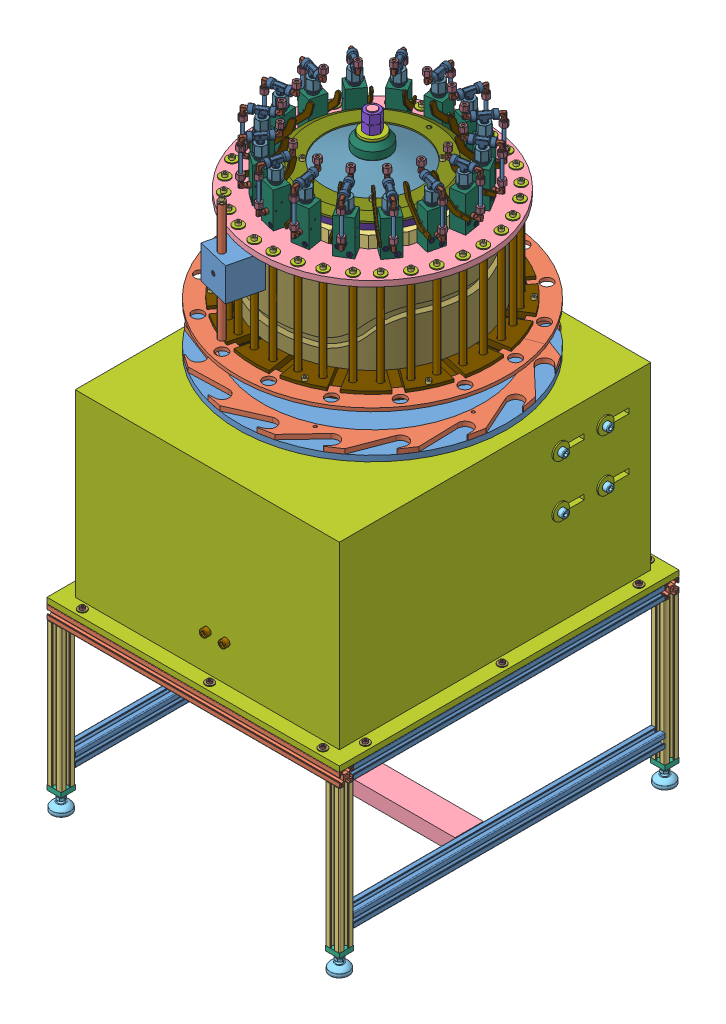
SolidWorks assembly Assieme_FINALE, configuration Default. Lengths in mm.
Overall size (1028.49 1273.72 1028.49).
701 component instances, 78 part files, 51 mates.
Components (placement in the parent):
- SupportoBase_Totale-2: SupportoBase_Totale [Default] at (4.0127 -14.4529 -3.9361) x (0 1 0) z (0 0 1) size (801.2 636.12 736.12)
  - Supporto_base_macchina-1: Supporto_base_macchina [Default] at origin size (378.2 636.12 736.12)
    - profilato_30x30_590-3: profilato_30x30_590 [Default] at (275.414 713.7262 -66.645) size (30 30 660)
    - profilato_30x30_590-5: profilato_30x30_590 [Default] at (275.414 123.7262 -66.645) size (30 30 660)
    - profilato_30x30_550-5: profilato_30x30_550 [Default] at (275.414 703.7262 -716.645) x (1 0 0) z (0 1 0) size (30 30 620)
    - profilato_30x30_550-6: profilato_30x30_550 [Default] at (275.414 703.7262 -26.645) x (1 0 0) z (0 1 0) size (30 30 620)
    - profilato_30x30_272-5: profilato_30x30_272 [Default] at (-16.586 123.7262 -716.645) x (0 0 1) z (-1 0 0) size (30 30 302)
    - profilato_30x30_272-6: profilato_30x30_272 [Default] at (-16.586 713.7262 -716.645) x (0 0 1) z (-1 0 0) size (30 30 302)
    - profilato_30x30_272-7: profilato_30x30_272 [Default] at (235.414 123.7262 -26.645) x (0 0 -1) z (1 0 0) size (30 30 302)
    - profilato_30x30_272-8: profilato_30x30_272 [Default] at (-16.586 713.7262 -26.645) x (0 0 1) z (-1 0 0) size (30 30 302)
    - profilo_U_60x30_490_supporto_base_macchina-1: profilo_U_60x30_490_supporto_base_macchina [Default] at (15.1 707.7262 -323.6583) x (0 0 1) z (0 -1 0) size (60 30 569)
    - profilato_30x30_590-6: profilato_30x30_590 [Default] at (3.414 123.7262 -66.645) size (30 30 660)
    - profilato_30x30_590-7: profilato_30x30_590 [Default] at (3.414 713.7262 -676.645) x (-1 0 0) z (0 0 -1) size (30 30 660)
    - 6322125-1: 6322125 [Default] at (-85.2818 713.7262 -26.645) x (0 0 -1) z (1 0 0) size (40 40 71.2)
    - 6322125-2: 6322125 [Default] at (-85.2818 713.7262 -716.645) x (0 0 -1) z (1 0 0) size (40 40 71.2)
    - 6322125-3: 6322125 [Default] at (-85.2818 123.7262 -26.645) x (0 -0.924225 -0.381849) z (1 0 0) size (40 40 71.2)
    - 6322125-4: 6322125 [Default] at (-85.2818 123.7262 -716.645) x (0 0 -1) z (1 0 0) size (40 40 71.2)
    - tappo_filettato_Supporto_base_macchina-1: tappo_filettato_Supporto_base_macchina [Default] at (-41.586 123.7262 -26.645) x (0 0 1) z (-1 0 0) size (30 30 10.37)
    - tappo_filettato_Supporto_base_macchina-2: tappo_filettato_Supporto_base_macchina [Default] at (-41.586 123.7262 -716.645) x (0 0 1) z (-1 0 0) size (30 30 10.37)
    - tappo_filettato_Supporto_base_macchina-3: tappo_filettato_Supporto_base_macchina [Default] at (-41.586 713.7262 -716.645) x (0 0 1) z (-1 0 0) size (30 30 10.37)
    - tappo_filettato_Supporto_base_macchina-4: tappo_filettato_Supporto_base_macchina [Default] at (-51.586 713.7262 -26.645) x (0 0 -1) z (1 0 0) size (30 30 10.37)
  - assieme_base-1: assieme_base [Default] at (466.8009 1138.7262 -472.0974) x (0 0 -1) z (0 -1 0) size (720 423 620)
    - Supporto di Base per macchina-1: Supporto di Base per macchina [Default] at (-460.4524 -176.3869 1030) size (720 403 620)
    - canotto di supporto-1: canotto di supporto [Default] at (-100.4524 134.8265 740) x (0 1 0) z (-0.866025 0 0.5) size (220 238 238)
    - m10 35mm-7: m10 35mm [ISO 4762 M10 x 35 - 35N] at (4.5476 246.6131 740) x (0 -1 0) z (1 0 0) size (45 16 16)
    - m10 35mm-8: m10 35mm [ISO 4762 M10 x 35 - 35N] at (-47.9524 246.6131 649.0673) x (0 -1 0) z (0.5 0 -0.866025) size (45 16 16)
    - m10 35mm-9: m10 35mm [ISO 4762 M10 x 35 - 35N] at (-152.9524 246.6131 649.0673) x (0 -1 0) z (-0.5 0 -0.866025) size (45 16 16)
    - m10 35mm-10: m10 35mm [ISO 4762 M10 x 35 - 35N] at (-205.4524 246.6131 740) x (0 -1 0) z (-1 0 0) size (45 16 16)
    - m10 35mm-11: m10 35mm [ISO 4762 M10 x 35 - 35N] at (-152.9524 246.6131 830.9327) x (0 -1 0) z (-0.5 0 0.866025) size (45 16 16)
    - m10 35mm-12: m10 35mm [ISO 4762 M10 x 35 - 35N] at (-47.9524 246.6131 830.9327) x (0 -1 0) z (0.5 0 0.866025) size (45 16 16)
    - Traversa di blocco albero-1: Traversa di blocco albero [Default] at (-100.4524 -86.3869 772.5) size (644 42 65)
    - m10 35mm-13: m10 35mm [ISO 4762 M10 x 35 - 35N] at (239.5476 -86.3869 760) x (-1 0 0) z (0 -1 0) size (45 16 16)
    - m10 35mm-16: m10 35mm [ISO 4762 M10 x 35 - 35N] at (239.5476 -86.3869 720) x (-1 0 0) z (0 -1 0) size (45 16 16)
    - m10 35mm-17: m10 35mm [ISO 4762 M10 x 35 - 35N] at (-440.4524 -86.3869 720) x (1 0 0) z (0 1 0) size (45 16 16)
    - m10 35mm-18: m10 35mm [ISO 4762 M10 x 35 - 35N] at (-440.4524 -86.3869 760) x (1 0 0) z (0 1 0) size (45 16 16)
  - DadoT-2: DadoT [Default] at (288.4104 668.7262 -716.645) x (0 0 -1) z (0 -1 0) size (16.5 6 8)
  - DadoT-9: DadoT [Default] at (288.4104 668.7262 -26.645) x (0 0 -1) z (0 -1 0) size (16.5 6 8)
  - DadoT-10: DadoT [Default] at (288.6104 713.7262 -661.645) x (0 1 0) z (0 0 -1) size (16.5 6 8)
  - DadoT-11: DadoT [Default] at (288.6104 713.7262 -371.645) x (0 1 0) z (0 0 -1) size (16.5 6 8)
  - DadoT-12: DadoT [Default] at (288.6104 713.7262 -81.645) x (0 1 0) z (0 0 -1) size (16.5 6 8)
  - DadoT-13: DadoT [Default] at (288.6104 123.7262 -661.645) x (0 1 0) z (0 0 -1) size (16.5 6 8)
  - DadoT-15: DadoT [Default] at (288.6104 123.7262 -371.645) x (0 1 0) z (0 0 -1) size (16.5 6 8)
  - DadoT-17: DadoT [Default] at (288.6104 123.7262 -81.645) x (0 1 0) z (0 0 -1) size (16.5 6 8)
  - RosettaM6-1: RosettaM6 [Washer ISO 7093 - 6] at (302.414 713.7262 -661.645) x (-1 0 0) z (0 0 1) size (1.6 18 18)
  - ViteM6-20-1: ViteM6-20 [ISO 4762 M6 x 20 - 20S] at (308.414 713.7262 -661.645) x (-1 0 0) z (0 0 1) size (26 10 10)
  - RosettaM6-2: RosettaM6 [Washer ISO 7093 - 6] at (302.414 668.7262 -716.645) x (-1 0 0) z (0 0 1) size (1.6 18 18)
  - ViteM6-20-2: ViteM6-20 [ISO 4762 M6 x 20 - 20S] at (308.414 668.7262 -716.645) x (-1 0 0) z (0 0 1) size (26 10 10)
  - RosettaM6-3: RosettaM6 [Washer ISO 7093 - 6] at (302.414 713.7262 -371.645) x (-1 0 0) z (0 0 1) size (1.6 18 18)
  - RosettaM6-4: RosettaM6 [Washer ISO 7093 - 6] at (302.414 713.7262 -81.645) x (-1 0 0) z (0 0 1) size (1.6 18 18)
  - ViteM6-20-3: ViteM6-20 [ISO 4762 M6 x 20 - 20S] at (308.414 713.7262 -371.645) x (-1 0 0) z (0 0 1) size (26 10 10)
  - ViteM6-20-4: ViteM6-20 [ISO 4762 M6 x 20 - 20S] at (308.414 713.7262 -81.645) x (-1 0 0) z (0 0 1) size (26 10 10)
  - RosettaM6-5: RosettaM6 [Washer ISO 7093 - 6] at (302.414 123.7262 -661.645) x (-1 0 0) z (0 0 1) size (1.6 18 18)
  - ViteM6-20-5: ViteM6-20 [ISO 4762 M6 x 20 - 20S] at (308.414 123.7262 -661.645) x (-1 0 0) z (0 0 1) size (26 10 10)
  - RosettaM6-6: RosettaM6 [Washer ISO 7093 - 6] at (302.414 123.7262 -371.645) x (-1 0 0) z (0 0 1) size (1.6 18 18)
  - RosettaM6-7: RosettaM6 [Washer ISO 7093 - 6] at (302.414 123.7262 -81.645) x (-1 0 0) z (0 0 1) size (1.6 18 18)
  - ViteM6-20-6: ViteM6-20 [ISO 4762 M6 x 20 - 20S] at (308.414 123.7262 -371.645) x (-1 0 0) z (0 0 1) size (26 10 10)
  - ViteM6-20-7: ViteM6-20 [ISO 4762 M6 x 20 - 20S] at (308.414 123.7262 -81.645) x (-1 0 0) z (0 0 1) size (26 10 10)
  - ViteM6-20-8: ViteM6-20 [ISO 4762 M6 x 20 - 20S] at (308.414 398.7262 -716.645) x (-1 0 0) z (0 0 1) size (26 10 10)
  - RosettaM6-8: RosettaM6 [Washer ISO 7093 - 6] at (302.414 398.7262 -716.645) x (-1 0 0) z (0 0 1) size (1.6 18 18)
  - DadoT-19: DadoT [Default] at (288.4104 398.7262 -716.645) x (0 0 -1) z (0 -1 0) size (16.5 6 8)
  - DadoT-20: DadoT [Default] at (288.4104 158.7262 -716.645) x (0 0 -1) z (0 -1 0) size (16.5 6 8)
  - RosettaM6-9: RosettaM6 [Washer ISO 7093 - 6] at (302.414 158.7262 -716.645) x (-1 0 0) z (0 0 1) size (1.6 18 18)
  - ViteM6-20-9: ViteM6-20 [ISO 4762 M6 x 20 - 20S] at (308.414 158.7262 -716.645) x (-1 0 0) z (0 0 1) size (26 10 10)
  - DadoT-21: DadoT [Default] at (288.4104 668.7262 -26.645) x (0 0 -1) z (0 -1 0) size (16.5 6 8)
  - RosettaM6-10: RosettaM6 [Washer ISO 7093 - 6] at (302.414 668.7262 -26.645) x (-1 0 0) z (0 0 1) size (1.6 18 18)
  - ViteM6-20-10: ViteM6-20 [ISO 4762 M6 x 20 - 20S] at (308.414 668.7262 -26.645) x (-1 0 0) z (0 0 1) size (26 10 10)
  - DadoT-22: DadoT [Default] at (288.4104 158.7262 -26.645) x (0 0 -1) z (0 -1 0) size (16.5 6 8)
  - RosettaM6-11: RosettaM6 [Washer ISO 7093 - 6] at (302.414 158.7262 -26.645) x (-1 0 0) z (0 0 1) size (1.6 18 18)
  - ViteM6-20-11: ViteM6-20 [ISO 4762 M6 x 20 - 20S] at (308.414 158.7262 -26.645) x (-1 0 0) z (0 0 1) size (26 10 10)
  - ViteM6-20-12: ViteM6-20 [ISO 4762 M6 x 20 - 20S] at (308.414 398.7262 -26.645) x (-1 0 0) z (0 0 1) size (26 10 10)
  - RosettaM6-12: RosettaM6 [Washer ISO 7093 - 6] at (302.414 398.7262 -26.645) x (-1 0 0) z (0 0 1) size (1.6 18 18)
  - DadoT-23: DadoT [Default] at (288.4104 398.7262 -26.645) x (0 0 -1) z (0 -1 0) size (16.5 6 8)
- motoriduttore-1: motoriduttore [Default] at (-164.7135 275.9611 -1137.0941) x (0 0 1) z (-1 0 0) size (200 160 175)
- Assieme_Riduttore-1: Assieme_Riduttore [Default] at (-58.5438 520.923 -522.9431) x (0 1 0) z (-0.993104 0 -0.117237) size (226 168.82 169.04)
  - AlberoRiduttore-1: AlberoRiduttore [Default] at (-61.6906 7.4655 211) size (201 29 29)
  - linguetta_uni6604_b_8x7x50-1: linguetta_uni6604_b_8x7x50 [Default] at (-116.7419 7.4655 226) x (1 0 0) z (0 1 0) size (50 7 8)
  - linguetta_uni6604_b_8x7x35-1: linguetta_uni6604_b_8x7x35 [Default] at (-33.7419 7.4655 226.5) x (1 0 0) z (0 1 0) size (35 7 8)
  - linguetta_uni6604_b_8x7x35-2: linguetta_uni6604_b_8x7x35 [Default] at (41.2581 7.4655 226.5) x (1 0 0) z (0 1 0) size (35 7 8)
  - ASSIEME-LASS-90-VERS-B-O-25-3D.step-1: ASSIEME-LASS-90-VERS-B-O-25-3D.step [Default] at (-111.3519 -70.5563 279.3493) x (-1 0 0) z (0 0.707107 -0.707107) size (64.28 105 105)
  - Rondella di fermo-1: Rondella di fermo [Default] at (-122.7419 7.4655 211) x (0 0.707107 -0.707107) z (-1 0 0) size (36 36 3)
  - M8 25 mm-1: M8 25 mm [ISO 4762 M8 x 25 - 25N] at (92.2581 7.4655 211) x (-1 0 0) z (0 1 0) size (33 13 13)
  - M8 25 mm-2: M8 25 mm [ISO 4762 M8 x 25 - 25N] at (-133.7419 7.4655 211) x (1 0 0) z (0 -0.707107 0.707107) size (33 13 13)
  - M6 16mm-3: M6 16mm [ISO 4762 M6 x 16 - 16N] at (-44.8119 40.5589 196.8286) x (-1 0 0) z (0 0.935687 0.352831) size (22 10 10)
  - M6 16mm-14: M6 16mm [ISO 4762 M6 x 16 - 16N] at (-44.8119 11.7394 175.2546) x (-1 0 0) z (0 0.773404 -0.633913) size (22 10 10)
  - M6 16mm-15: M6 16mm [ISO 4762 M6 x 16 - 16N] at (-44.8119 -21.354 189.426) x (-1 0 0) z (0 -0.162283 -0.986744) size (22 10 10)
  - M6 16mm-16: M6 16mm [ISO 4762 M6 x 16 - 16N] at (-44.8119 -25.6279 225.1714) x (-1 0 0) z (0 -0.935687 -0.352831) size (22 10 10)
  - M6 16mm-17: M6 16mm [ISO 4762 M6 x 16 - 16N] at (-44.8119 3.1916 246.7454) x (-1 0 0) z (0 -0.773404 0.633913) size (22 10 10)
  - M6 16mm-18: M6 16mm [ISO 4762 M6 x 16 - 16N] at (-44.8119 36.285 232.574) x (-1 0 0) z (0 0.162283 0.986744) size (22 10 10)
  - Parte1^Assieme_Riduttore-1: Parte1^Assieme_Riduttore [Default] at origin (virtual)
  - ruota dentata m22-4: ruota dentata m22 [Chain wheel ISO - 22Z 10A-1 --22SA36.0N] at (-59.7419 7.4655 211) x (1 0 0) z (0 -0.599278 0.800541) size (8.93 120.13 121.23)
  - Rondella di fermo-2: Rondella di fermo [Default] at (84.2581 7.4655 211) x (0 0 1) z (-1 0 0) size (36 36 3)
- M10 50mm-1: M10 50mm [ISO 4762 M10 x 50 - 50N] at (-121.7135 603.4611 -513.0941) x (-1 0 0) z (0 -0.924225 -0.381849) size (60 16 16)
- M10 50mm-2: M10 50mm [ISO 4762 M10 x 50 - 50N] at (-121.7135 492.4611 -513.0941) x (-1 0 0) z (0 0 1) size (60 16 16)
- M10 50mm-5: M10 50mm [ISO 4762 M10 x 50 - 50N] at (-121.7135 603.4611 -608.0941) x (-1 0 0) z (0 0 1) size (60 16 16)
- M10 50mm-4: M10 50mm [ISO 4762 M10 x 50 - 50N] at (-121.7135 492.4611 -608.0941) x (-1 0 0) z (0 0 1) size (60 16 16)
- DADO M10-9: DADO M10 [ISO - 4033 - M10 - W - N] at (-174.0135 603.4611 -608.0941) x (0 0 1) z (-1 0 0) size (16 18.48 9.3)
- DADO M10-8: DADO M10 [ISO - 4033 - M10 - W - N] at (-174.0135 603.4611 -513.0941) x (0 0 1) z (-1 0 0) size (16 18.48 9.3)
- DADO M10-7: DADO M10 [ISO - 4033 - M10 - W - N] at (-174.0135 492.4611 -608.0941) x (0 0 1) z (-1 0 0) size (16 18.48 9.3)
- DADO M10-10: DADO M10 [ISO - 4033 - M10 - W - N] at (-174.0135 492.4611 -513.0941) x (0 0 1) z (-1 0 0) size (16 18.48 9.3)
- rondella M10-9: rondella M10 [Washer ISO 7094 - 10] at (-134.7135 603.4611 -513.0941) x (-1 0 0) z (0 0.924225 0.381849) size (3 34 34)
- rondella M10-10: rondella M10 [Washer ISO 7094 - 10] at (-134.7135 492.4611 -513.0941) x (-1 0 0) z (0 0 1) size (3 34 34)
- rondella M10-12: rondella M10 [Washer ISO 7094 - 10] at (-134.7135 492.4611 -608.0941) x (-1 0 0) z (0 0 1) size (3 34 34)
- rondella M10-11: rondella M10 [Washer ISO 7094 - 10] at (-134.7135 603.4611 -608.0941) x (-1 0 0) z (0 0 1) size (3 34 34)
- catena_maschio-1: catena_maschio [Default] at (-321.9473 463.4961 -580.6395) x (-0.810007 0 0.58642) z (0 1 0) size (28.67 12.73 20.3)
- catena_femmina-1: catena_femmina [Default] at (-334.299 463.4961 -567.4631) x (0.810007 0 -0.58642) z (0 1 0) size (30.04 14.2 13.87)
  - ansi_50_02-1: ansi_50_02 [Default] at (17.7318 3.4296 0) x (1 0 0) z (0 0 -1) size (30.04 14.2 13.87)
  - ansi_50_03-1: ansi_50_03 [Default] at (17.7318 3.4296 -0.11) x (1 0 0) z (0 0 -1) size (10.16 10.16 9.46)
  - ansi_50_04-1: ansi_50_04 [Default] at (17.7318 3.4296 0.11) x (1 0 0) z (0 0 -1) size (10.16 10.16 9.46)
- rondella M8-1: rondella M8 [ISO 10673-9.3-S] at (-394.7135 376.9611 -360.5811) x (0 -1 0) z (-1 0 0) size (2 18 18)
- rondella M8-2: rondella M8 [ISO 10673-9.3-S] at (-394.7135 376.9611 -390.5811) x (0 -1 0) z (-1 0 0) size (2 18 18)
- M8 25 mm-1: M8 25 mm [ISO 4762 M8 x 25 - 25N] at (-394.7135 368.9611 -390.5811) x (0 1 0) z (0.5 0 0.866025) size (33 13 13)
- M8 25 mm-2: M8 25 mm [ISO 4762 M8 x 25 - 25N] at (-394.7135 366.9611 -360.5811) x (0 1 0) z (-0.5 0 -0.866025) size (33 13 13)
- assieme parte rotante-2: assieme parte rotante [Default] at (-8.3038 623.9178 -528.0599) x (0 1 0) z (-0.913062 0 0.407822) size (749.63 778.63 778.63)
  - albero rotazione piatti-1: albero rotazione piatti [Default] at (60.413 18.3637 415) size (415 200 200)
  - seger 100mm-2: seger 100mm [KS 1336 E - 100] at (-146.4567 18.3637 415) x (0 0 -1) z (1 0 0) size (107.55 112.98 3)
  - SKF - 6020 - 20,DE,NC,20_68-1: SKF - 6020 - 20,DE,NC,20_68 [SKF - 6020 - 20,DE,NC,20_68] at (-131.4567 18.3637 415) x (1 0 0) z (0 -0.434476 -0.900684) size (24 150 150)
  - calettatore d95-1: calettatore d95 [Default] at (-173.8867 18.3637 415) size (39.5 135 135)
  - Chain wheel ISO - 50Z 10A-1-1: Chain wheel ISO - 50Z 10A-1 [Chain wheel ISO - 50Z 10A-1 --50SB120H25L95.0N] at (-164.8867 18.3637 415) size (28.93 262.06 262.51)
  - Disco supporto montaggio e Colonne-1: Disco supporto montaggio e Colonne [Default] at (204.0433 18.3637 415) x (0 -0.866025 -0.5) z (1 0 0) size (499.6 499.6 29)
  - SKF - 6020 - 20,DE,NC,20_68-2: SKF - 6020 - 20,DE,NC,20_68 [SKF - 6020 - 20,DE,NC,20_68] at (62.0433 18.3637 415) x (1 0 0) z (0 -0.432628 -0.901573) size (24 150 150)
  - piatto rotante porta tappi-1: piatto rotante porta tappi [Default] at (99.0433 18.3637 415) x (0 0 -1) z (1 0 0) size (570 570 20.57)
  - disco trasportatore tappi 31-1: disco trasportatore tappi 31 [Default] at (111.0433 18.3637 415) x (0 0.5 -0.866025) z (1 0 0) size (570 570 10.42)
  - Distributore Rotante-1: Distributore Rotante [Default] at (425.0433 18.3637 415) x (0 0.130526 -0.991445) z (1 0 0) size (310 310 25.54)
  - disco trascinato porta distributore vuoto-1: disco trascinato porta distributore vuoto [Default] at (400.0433 18.3637 415) x (0 -0.130526 0.991445) z (-1 0 0) size (480 480 50)
  - m12 35mm-1: m12 35mm [ISO 4762 M12 x 35 - 35N] at (376.0433 -45.1046 366.2991) x (1 0 0) z (0 -0.5 0.866025) size (47 18 18)
  - m12 90mm-3: m12 90mm [ISO 4762 M12 x 90 - 90N] at (203.0433 -21.6363 345.718) x (-1 0 0) z (0 -0.5 0.866025) size (102 18 18)
  - rondella M6-90: rondella M6 [Washer ISO 7094 - 6] at (99.0433 -101.6363 207.1539) x (1 0 0) z (0 -1 0) size (2 22 22)
  - M6 20mm-1: M6 20mm [ISO 4762 M6 x 20 - 20N] at (91.0433 -101.6363 207.1539) x (1 0 0) z (0 0.5 0.866025) size (26 10 10)
  - m12 35mm-2: m12 35mm [ISO 4762 M12 x 35 - 35N] at (376.0433 28.8058 335.6844) x (1 0 0) z (0 -1 0) size (47 18 18)
  - m12 35mm-3: m12 35mm [ISO 4762 M12 x 35 - 35N] at (376.0433 92.2741 384.3853) x (1 0 0) z (0 -0.5 -0.866025) size (47 18 18)
  - m12 35mm-4: m12 35mm [ISO 4762 M12 x 35 - 35N] at (376.0433 81.832 463.7009) x (1 0 0) z (0 0.5 -0.866025) size (47 18 18)
  - m12 35mm-5: m12 35mm [ISO 4762 M12 x 35 - 35N] at (376.0433 7.9216 494.3156) x (1 0 0) z (0 1 0) size (47 18 18)
  - m12 35mm-6: m12 35mm [ISO 4762 M12 x 35 - 35N] at (376.0433 -55.5467 445.6147) x (1 0 0) z (0 0.5 0.866025) size (47 18 18)
  - rondella M6-91: rondella M6 [Washer ISO 7094 - 6] at (99.0433 138.3637 207.1539) x (1 0 0) z (0 -0.5 -0.866025) size (2 22 22)
  - rondella M6-92: rondella M6 [Washer ISO 7094 - 6] at (99.0433 258.3637 415) x (1 0 0) z (0 0.5 -0.866025) size (2 22 22)
  - rondella M6-93: rondella M6 [Washer ISO 7094 - 6] at (99.0433 138.3637 622.8461) x (1 0 0) z (0 1 0) size (2 22 22)
  - rondella M6-94: rondella M6 [Washer ISO 7094 - 6] at (99.0433 -101.6363 622.8461) x (1 0 0) z (0 0.5 0.866025) size (2 22 22)
  - rondella M6-95: rondella M6 [Washer ISO 7094 - 6] at (99.0433 -221.6363 415) x (1 0 0) z (0 -0.5 0.866025) size (2 22 22)
  - M6 20mm-2: M6 20mm [ISO 4762 M6 x 20 - 20N] at (91.0433 138.3637 207.1539) x (1 0 0) z (0 -0.5 0.866025) size (26 10 10)
  - M6 20mm-3: M6 20mm [ISO 4762 M6 x 20 - 20N] at (91.0433 258.3637 415) x (1 0 0) z (0 -1 0) size (26 10 10)
  - M6 20mm-4: M6 20mm [ISO 4762 M6 x 20 - 20N] at (91.0433 138.3637 622.8461) x (1 0 0) z (0 -0.5 -0.866025) size (26 10 10)
  - M6 20mm-5: M6 20mm [ISO 4762 M6 x 20 - 20N] at (91.0433 -101.6363 622.8461) x (1 0 0) z (0 0.5 -0.866025) size (26 10 10)
  - M6 20mm-6: M6 20mm [ISO 4762 M6 x 20 - 20N] at (91.0433 -221.6363 415) x (1 0 0) z (0 1 0) size (26 10 10)
  - m12 90mm-4: m12 90mm [ISO 4762 M12 x 90 - 90N] at (203.0433 58.3637 345.718) x (-1 0 0) z (0 -1 0) size (102 18 18)
  - m12 90mm-5: m12 90mm [ISO 4762 M12 x 90 - 90N] at (203.0433 98.3637 415) x (-1 0 0) z (0 -0.5 -0.866025) size (102 18 18)
  - m12 90mm-6: m12 90mm [ISO 4762 M12 x 90 - 90N] at (203.0433 58.3637 484.282) x (-1 0 0) z (0 0.5 -0.866025) size (102 18 18)
  - m12 90mm-7: m12 90mm [ISO 4762 M12 x 90 - 90N] at (203.0433 -21.6363 484.282) x (-1 0 0) z (0 1 0) size (102 18 18)
  - m12 90mm-8: m12 90mm [ISO 4762 M12 x 90 - 90N] at (203.0433 -61.6363 415) x (-1 0 0) z (0 0.5 0.866025) size (102 18 18)
  - asta scorrimento carello-1: asta scorrimento carello [Default] at (287.5433 70.1437 197.9013) x (0 0 -1) z (1 0 0) size (12 12 225)
  - rondella M6-74: rondella M6 [Washer ISO 7094 - 6] at (175.0433 70.1437 197.9013) x (1 0 0) z (0 -1 0) size (2 22 22)
  - M6 16mm-1: M6 16mm [ISO 4762 M6 x 16 - 16N] at (167.0433 70.1437 197.9013) size (22 10 10)
  - M6 16mm-2: M6 16mm [ISO 4762 M6 x 16 - 16N] at (408.0433 70.1437 197.9013) x (-1 0 0) z (0 0 -1) size (22 10 10)
  - rondella M6-96: rondella M6 [Washer ISO 7094 - 6] at (400.0433 70.1437 197.9013) x (-1 0 0) z (0 1 0) size (2 22 22)
  - rondella M6-112: rondella M6 [Washer ISO 7094 - 6] at (175.0433 24.5373 191.8971) x (1 0 0) z (0 -0.965926 -0.258819) size (2 22 22)
  - M6 16mm-3: M6 16mm [ISO 4762 M6 x 16 - 16N] at (167.0433 24.5373 191.8971) x (1 0 0) z (0 0.258819 -0.965926) size (22 10 10)
  - asta scorrimento carello-2: asta scorrimento carello [Default] at (287.5433 24.5373 191.8971) x (0 0.258819 -0.965926) z (-1 0 0) size (12 12 225)
  - rondella M6-128: rondella M6 [Washer ISO 7094 - 6] at (400.0433 24.5373 191.8971) x (-1 0 0) z (0 0.965926 0.258819) size (2 22 22)
  - M6 16mm-4: M6 16mm [ISO 4762 M6 x 16 - 16N] at (408.0433 24.5373 191.8971) x (-1 0 0) z (0 -0.258819 0.965926) size (22 10 10)
  - AssiemeValvola-1: AssiemeValvola [Default] at (515.3257 103.3637 267.7757) x (0 -0.5 0.866025) z (0 0.866025 0.5) size (90.26 138.63 38)
    - RaccordoT-1: RaccordoT [Default] at origin size (43 29.75 16.5)
    - Raccordo a L-1: Raccordo a L [Default] at (-30 0 0) x (0 -1 0) z (0 0 -1) size (28.34 25.51 14.01)
      - 1809_06_10_01-1: 1809_06_10_01 [Default] at origin size (22.49 23 10)
      - 1809_06_10_02-1: 1809_06_10_02 [Default] at origin size (6.5 8.5 8.5)
      - 1809_06_10_03-1: 1809_06_10_03 [Default] at origin size (11.02 15.01 14.01)
    - Raccordo a L-2: Raccordo a L [Default] at (30 0 0) x (0 1 0) z (0 0 -1) size (28.34 25.51 14.01)
      - 1809_06_10_01-1: 1809_06_10_01 [Default] at origin size (22.49 23 10)
      - 1809_06_10_02-1: 1809_06_10_02 [Default] at origin size (6.5 8.5 8.5)
      - 1809_06_10_03-1: 1809_06_10_03 [Default] at origin size (11.02 15.01 14.01)
    - TappoChiusura-1: TappoChiusura [Default] at (0 -32 0) x (0 -1 0) z (0 0 1) size (38.28 26.74 26.74)
    - CorpoValvola-1: CorpoValvola [Default] at (-15 -115.2824 0) size (30 75 34)
    - Raccordo a L-3: Raccordo a L [Default] at (-30 -88.2824 0) x (0 1 0) z (0 0 1) size (28.34 25.51 14.01)
      - 1809_06_10_01-1: 1809_06_10_01 [Default] at origin size (22.49 23 10)
      - 1809_06_10_02-1: 1809_06_10_02 [Default] at origin size (6.5 8.5 8.5)
      - 1809_06_10_03-1: 1809_06_10_03 [Default] at origin size (11.02 15.01 14.01)
    - Spina_3x38-1: Spina_3x38 [Default] at (0 -68.2824 -21) x (-1 0 0) z (0 0 1) size (3 3 38)
    - Spina_3x38-2: Spina_3x38 [Default] at (-10 -80.2824 -21) x (0.996193 0.087174 0) z (0 0 1) size (3 3 38)
    - M5 40mm-3: M5 40mm [ISO 4762 M5 x 40 - 40N] at (-14.6 -108.7824 9) size (45 8.5 8.5)
    - M5 40mm-2: M5 40mm [ISO 4762 M5 x 40 - 40N] at (-14.6 -96.7824 -9) size (45 8.5 8.5)
    - LevaValvola-1: LevaValvola [Default] at (-24.507 -86.571 -17) x (0.996193 0.087174 0) z (0 0 1) size (77.55 60.2 4)
    - Tubo-1: Tubo [Default] at (-30 -15.9665 0) x (1 0 0) z (0 -1 0) size (6 6 56.4)
  - M6 16mm-5: M6 16mm [ISO 4762 M6 x 16 - 16N] at (167.0433 -16.8778 194.6116) x (1 0 0) z (0 0.382683 0.92388) size (22 10 10)
  - M6 16mm-6: M6 16mm [ISO 4762 M6 x 16 - 16N] at (167.0433 -98.5342 224.874) x (1 0 0) z (0 0.707107 0.707107) size (22 10 10)
  - M6 16mm-7: M6 16mm [ISO 4762 M6 x 16 - 16N] at (167.0433 -162.3939 284.0814) x (1 0 0) z (0 0.92388 0.382683) size (22 10 10)
  - M6 16mm-8: M6 16mm [ISO 4762 M6 x 16 - 16N] at (167.0433 -198.735 363.22) x (1 0 0) z (0 1 0) size (22 10 10)
  - M6 16mm-9: M6 16mm [ISO 4762 M6 x 16 - 16N] at (167.0433 -202.0247 450.2415) x (1 0 0) z (0 0.92388 -0.382683) size (22 10 10)
  - M6 16mm-10: M6 16mm [ISO 4762 M6 x 16 - 16N] at (167.0433 -171.7623 531.8979) x (1 0 0) z (0 0.707107 -0.707107) size (22 10 10)
  - M6 16mm-11: M6 16mm [ISO 4762 M6 x 16 - 16N] at (167.0433 -112.5549 595.7576) x (1 0 0) z (0 0.382683 -0.92388) size (22 10 10)
  - M6 16mm-12: M6 16mm [ISO 4762 M6 x 16 - 16N] at (167.0433 -33.4163 632.0987) x (1 0 0) z (0 0 -1) size (22 10 10)
  - M6 16mm-13: M6 16mm [ISO 4762 M6 x 16 - 16N] at (167.0433 53.6052 635.3884) x (1 0 0) z (0 -0.382683 -0.92388) size (22 10 10)
  - M6 16mm-14: M6 16mm [ISO 4762 M6 x 16 - 16N] at (167.0433 135.2616 605.126) x (1 0 0) z (0 -0.707107 -0.707107) size (22 10 10)
  - M6 16mm-15: M6 16mm [ISO 4762 M6 x 16 - 16N] at (167.0433 199.1213 545.9186) x (1 0 0) z (0 -0.92388 -0.382683) size (22 10 10)
  - M6 16mm-16: M6 16mm [ISO 4762 M6 x 16 - 16N] at (167.0433 235.4624 466.78) x (1 0 0) z (0 -1 0) size (22 10 10)
  - M6 16mm-17: M6 16mm [ISO 4762 M6 x 16 - 16N] at (167.0433 238.7521 379.7585) x (1 0 0) z (0 -0.92388 0.382683) size (22 10 10)
  - M6 16mm-18: M6 16mm [ISO 4762 M6 x 16 - 16N] at (167.0433 208.4897 298.1021) x (1 0 0) z (0 -0.707107 0.707107) size (22 10 10)
  - M6 16mm-19: M6 16mm [ISO 4762 M6 x 16 - 16N] at (167.0433 149.2823 234.2424) x (1 0 0) z (0 -0.382683 0.92388) size (22 10 10)
  - rondella M6-75: rondella M6 [Washer ISO 7094 - 6] at (175.0433 -16.8778 194.6116) x (1 0 0) z (0 -0.92388 0.382683) size (2 22 22)
  - rondella M6-76: rondella M6 [Washer ISO 7094 - 6] at (175.0433 -98.5342 224.874) x (1 0 0) z (0 -0.707107 0.707107) size (2 22 22)
  - rondella M6-77: rondella M6 [Washer ISO 7094 - 6] at (175.0433 -162.3939 284.0814) x (1 0 0) z (0 -0.382683 0.92388) size (2 22 22)
  - rondella M6-78: rondella M6 [Washer ISO 7094 - 6] at (175.0433 -198.735 363.22) size (2 22 22)
  - rondella M6-79: rondella M6 [Washer ISO 7094 - 6] at (175.0433 -202.0247 450.2415) x (1 0 0) z (0 0.382683 0.92388) size (2 22 22)
  - rondella M6-80: rondella M6 [Washer ISO 7094 - 6] at (175.0433 -171.7623 531.8979) x (1 0 0) z (0 0.707107 0.707107) size (2 22 22)
  - rondella M6-81: rondella M6 [Washer ISO 7094 - 6] at (175.0433 -112.5549 595.7576) x (1 0 0) z (0 0.92388 0.382683) size (2 22 22)
  - rondella M6-82: rondella M6 [Washer ISO 7094 - 6] at (175.0433 -33.4163 632.0987) x (1 0 0) z (0 1 0) size (2 22 22)
  - rondella M6-83: rondella M6 [Washer ISO 7094 - 6] at (175.0433 53.6052 635.3884) x (1 0 0) z (0 0.92388 -0.382683) size (2 22 22)
  - rondella M6-84: rondella M6 [Washer ISO 7094 - 6] at (175.0433 135.2616 605.126) x (1 0 0) z (0 0.707107 -0.707107) size (2 22 22)
  - rondella M6-85: rondella M6 [Washer ISO 7094 - 6] at (175.0433 199.1213 545.9186) x (1 0 0) z (0 0.382683 -0.92388) size (2 22 22)
  - rondella M6-86: rondella M6 [Washer ISO 7094 - 6] at (175.0433 235.4624 466.78) x (1 0 0) z (0 0 -1) size (2 22 22)
  - rondella M6-87: rondella M6 [Washer ISO 7094 - 6] at (175.0433 238.7521 379.7585) x (1 0 0) z (0 -0.382683 -0.92388) size (2 22 22)
  - rondella M6-88: rondella M6 [Washer ISO 7094 - 6] at (175.0433 208.4897 298.1021) x (1 0 0) z (0 -0.707107 -0.707107) size (2 22 22)
  - rondella M6-89: rondella M6 [Washer ISO 7094 - 6] at (175.0433 149.2823 234.2424) x (1 0 0) z (0 -0.92388 -0.382683) size (2 22 22)
  - asta scorrimento carello-3: asta scorrimento carello [Default] at (287.5433 -16.8778 194.6116) x (0 -0.382683 -0.92388) z (1 0 0) size (12 12 225)
  - asta scorrimento carello-4: asta scorrimento carello [Default] at (287.5433 -98.5342 224.874) x (0 -0.707107 -0.707107) z (1 0 0) size (12 12 225)
  - asta scorrimento carello-5: asta scorrimento carello [Default] at (287.5433 -162.3939 284.0814) x (0 -0.92388 -0.382683) z (1 0 0) size (12 12 225)
  - asta scorrimento carello-6: asta scorrimento carello [Default] at (287.5433 -198.735 363.22) x (0 -1 0) z (1 0 0) size (12 12 225)
  - asta scorrimento carello-7: asta scorrimento carello [Default] at (287.5433 -202.0247 450.2415) x (0 -0.92388 0.382683) z (1 0 0) size (12 12 225)
  - asta scorrimento carello-8: asta scorrimento carello [Default] at (287.5433 -171.7623 531.8979) x (0 -0.707107 0.707107) z (1 0 0) size (12 12 225)
  - asta scorrimento carello-9: asta scorrimento carello [Default] at (287.5433 -112.5549 595.7576) x (0 -0.382683 0.92388) z (1 0 0) size (12 12 225)
  - asta scorrimento carello-10: asta scorrimento carello [Default] at (287.5433 -33.4163 632.0987) x (0 0 1) z (1 0 0) size (12 12 225)
  - asta scorrimento carello-11: asta scorrimento carello [Default] at (287.5433 53.6052 635.3884) x (0 0.382683 0.92388) z (1 0 0) size (12 12 225)
  - asta scorrimento carello-12: asta scorrimento carello [Default] at (287.5433 135.2616 605.126) x (0 0.707107 0.707107) z (1 0 0) size (12 12 225)
  - asta scorrimento carello-13: asta scorrimento carello [Default] at (287.5433 199.1213 545.9186) x (0 0.92388 0.382683) z (1 0 0) size (12 12 225)
  - asta scorrimento carello-14: asta scorrimento carello [Default] at (287.5433 235.4624 466.78) x (0 1 0) z (1 0 0) size (12 12 225)
  - asta scorrimento carello-15: asta scorrimento carello [Default] at (287.5433 238.7521 379.7585) x (0 0.92388 -0.382683) z (1 0 0) size (12 12 225)
  - asta scorrimento carello-16: asta scorrimento carello [Default] at (287.5433 208.4897 298.1021) x (0 0.707107 -0.707107) z (1 0 0) size (12 12 225)
  - asta scorrimento carello-17: asta scorrimento carello [Default] at (287.5433 149.2823 234.2424) x (0 0.382683 -0.92388) z (1 0 0) size (12 12 225)
  - M6 16mm-20: M6 16mm [ISO 4762 M6 x 16 - 16N] at (408.0433 -16.8778 194.6116) x (-1 0 0) z (0 -0.382683 -0.92388) size (22 10 10)
  - M6 16mm-21: M6 16mm [ISO 4762 M6 x 16 - 16N] at (408.0433 -98.5342 224.874) x (-1 0 0) z (0 -0.707107 -0.707107) size (22 10 10)
  - M6 16mm-22: M6 16mm [ISO 4762 M6 x 16 - 16N] at (408.0433 -162.3939 284.0814) x (-1 0 0) z (0 -0.92388 -0.382683) size (22 10 10)
  - M6 16mm-23: M6 16mm [ISO 4762 M6 x 16 - 16N] at (408.0433 -198.735 363.22) x (-1 0 0) z (0 -1 0) size (22 10 10)
  - M6 16mm-24: M6 16mm [ISO 4762 M6 x 16 - 16N] at (408.0433 -202.0247 450.2415) x (-1 0 0) z (0 -0.92388 0.382683) size (22 10 10)
  - M6 16mm-25: M6 16mm [ISO 4762 M6 x 16 - 16N] at (408.0433 -171.7623 531.8979) x (-1 0 0) z (0 -0.707107 0.707107) size (22 10 10)
  - M6 16mm-26: M6 16mm [ISO 4762 M6 x 16 - 16N] at (408.0433 -112.5549 595.7576) x (-1 0 0) z (0 -0.382683 0.92388) size (22 10 10)
  - M6 16mm-27: M6 16mm [ISO 4762 M6 x 16 - 16N] at (408.0433 -33.4163 632.0987) x (-1 0 0) z (0 0 1) size (22 10 10)
  - M6 16mm-28: M6 16mm [ISO 4762 M6 x 16 - 16N] at (408.0433 53.6052 635.3884) x (-1 0 0) z (0 0.382683 0.92388) size (22 10 10)
  - M6 16mm-29: M6 16mm [ISO 4762 M6 x 16 - 16N] at (408.0433 135.2616 605.126) x (-1 0 0) z (0 0.707107 0.707107) size (22 10 10)
  - M6 16mm-30: M6 16mm [ISO 4762 M6 x 16 - 16N] at (408.0433 199.1213 545.9186) x (-1 0 0) z (0 0.92388 0.382683) size (22 10 10)
  - M6 16mm-31: M6 16mm [ISO 4762 M6 x 16 - 16N] at (408.0433 235.4624 466.78) x (-1 0 0) z (0 1 0) size (22 10 10)
  - M6 16mm-32: M6 16mm [ISO 4762 M6 x 16 - 16N] at (408.0433 238.7521 379.7585) x (-1 0 0) z (0 0.92388 -0.382683) size (22 10 10)
  - M6 16mm-33: M6 16mm [ISO 4762 M6 x 16 - 16N] at (408.0433 208.4897 298.1021) x (-1 0 0) z (0 0.707107 -0.707107) size (22 10 10)
  - M6 16mm-34: M6 16mm [ISO 4762 M6 x 16 - 16N] at (408.0433 149.2823 234.2424) x (-1 0 0) z (0 0.382683 -0.92388) size (22 10 10)
  - rondella M6-97: rondella M6 [Washer ISO 7094 - 6] at (400.0433 -16.8778 194.6116) x (-1 0 0) z (0 0.92388 -0.382683) size (2 22 22)
  - rondella M6-98: rondella M6 [Washer ISO 7094 - 6] at (400.0433 -98.5342 224.874) x (-1 0 0) z (0 0.707107 -0.707107) size (2 22 22)
  - rondella M6-99: rondella M6 [Washer ISO 7094 - 6] at (400.0433 -162.3939 284.0814) x (-1 0 0) z (0 0.382683 -0.92388) size (2 22 22)
  - rondella M6-100: rondella M6 [Washer ISO 7094 - 6] at (400.0433 -198.735 363.22) x (-1 0 0) z (0 0 -1) size (2 22 22)
  - rondella M6-101: rondella M6 [Washer ISO 7094 - 6] at (400.0433 -202.0247 450.2415) x (-1 0 0) z (0 -0.382683 -0.92388) size (2 22 22)
  - rondella M6-102: rondella M6 [Washer ISO 7094 - 6] at (400.0433 -171.7623 531.8979) x (-1 0 0) z (0 -0.707107 -0.707107) size (2 22 22)
  - rondella M6-103: rondella M6 [Washer ISO 7094 - 6] at (400.0433 -112.5549 595.7576) x (-1 0 0) z (0 -0.92388 -0.382683) size (2 22 22)
  - rondella M6-104: rondella M6 [Washer ISO 7094 - 6] at (400.0433 -33.4163 632.0987) x (-1 0 0) z (0 -1 0) size (2 22 22)
  - rondella M6-105: rondella M6 [Washer ISO 7094 - 6] at (400.0433 53.6052 635.3884) x (-1 0 0) z (0 -0.92388 0.382683) size (2 22 22)
  - rondella M6-106: rondella M6 [Washer ISO 7094 - 6] at (400.0433 135.2616 605.126) x (-1 0 0) z (0 -0.707107 0.707107) size (2 22 22)
  - rondella M6-107: rondella M6 [Washer ISO 7094 - 6] at (400.0433 199.1213 545.9186) x (-1 0 0) z (0 -0.382683 0.92388) size (2 22 22)
  - rondella M6-108: rondella M6 [Washer ISO 7094 - 6] at (400.0433 235.4624 466.78) x (-1 0 0) z (0 0 1) size (2 22 22)
  - rondella M6-109: rondella M6 [Washer ISO 7094 - 6] at (400.0433 238.7521 379.7585) x (-1 0 0) z (0 0.382683 0.92388) size (2 22 22)
  - rondella M6-110: rondella M6 [Washer ISO 7094 - 6] at (400.0433 208.4897 298.1021) x (-1 0 0) z (0 0.707107 0.707107) size (2 22 22)
  - rondella M6-111: rondella M6 [Washer ISO 7094 - 6] at (400.0433 149.2823 234.2424) x (-1 0 0) z (0 0.92388 0.382683) size (2 22 22)
  - rondella M6-113: rondella M6 [Washer ISO 7094 - 6] at (175.0433 -61.3104 206.5173) x (1 0 0) z (0 -0.991445 0.130526) size (2 22 22)
  - rondella M6-114: rondella M6 [Washer ISO 7094 - 6] at (175.0433 -135.0285 252.8771) x (1 0 0) z (0 -0.866025 0.5) size (2 22 22)
  - rondella M6-115: rondella M6 [Washer ISO 7094 - 6] at (175.0433 -185.3939 323.9186) x (1 0 0) z (0 -0.608761 0.793353) size (2 22 22)
  - rondella M6-116: rondella M6 [Washer ISO 7094 - 6] at (175.0433 -204.7392 408.8264) x (1 0 0) z (0 -0.258819 0.965926) size (2 22 22)
  - rondella M6-117: rondella M6 [Washer ISO 7094 - 6] at (175.0433 -190.119 494.6741) x (1 0 0) z (0 0.130526 0.991445) size (2 22 22)
  - rondella M6-118: rondella M6 [Washer ISO 7094 - 6] at (175.0433 -143.7592 568.3922) x (1 0 0) z (0 0.5 0.866025) size (2 22 22)
  - rondella M6-119: rondella M6 [Washer ISO 7094 - 6] at (175.0433 -72.7177 618.7576) x (1 0 0) z (0 0.793353 0.608761) size (2 22 22)
  - rondella M6-120: rondella M6 [Washer ISO 7094 - 6] at (175.0433 12.1901 638.1029) x (1 0 0) z (0 0.965926 0.258819) size (2 22 22)
  - rondella M6-121: rondella M6 [Washer ISO 7094 - 6] at (175.0433 98.0378 623.4827) x (1 0 0) z (0 0.991445 -0.130526) size (2 22 22)
  - rondella M6-122: rondella M6 [Washer ISO 7094 - 6] at (175.0433 171.7559 577.1229) x (1 0 0) z (0 0.866025 -0.5) size (2 22 22)
  - rondella M6-123: rondella M6 [Washer ISO 7094 - 6] at (175.0433 222.1213 506.0814) x (1 0 0) z (0 0.608761 -0.793353) size (2 22 22)
  - rondella M6-124: rondella M6 [Washer ISO 7094 - 6] at (175.0433 241.4666 421.1736) x (1 0 0) z (0 0.258819 -0.965926) size (2 22 22)
  - rondella M6-125: rondella M6 [Washer ISO 7094 - 6] at (175.0433 226.8464 335.3259) x (1 0 0) z (0 -0.130526 -0.991445) size (2 22 22)
  - rondella M6-126: rondella M6 [Washer ISO 7094 - 6] at (175.0433 180.4866 261.6078) x (1 0 0) z (0 -0.5 -0.866025) size (2 22 22)
  - rondella M6-127: rondella M6 [Washer ISO 7094 - 6] at (175.0433 109.4451 211.2424) x (1 0 0) z (0 -0.793353 -0.608761) size (2 22 22)
  - M6 16mm-35: M6 16mm [ISO 4762 M6 x 16 - 16N] at (167.0433 -61.3104 206.5173) x (1 0 0) z (0 -0.130526 -0.991445) size (22 10 10)
  - M6 16mm-36: M6 16mm [ISO 4762 M6 x 16 - 16N] at (167.0433 -135.0285 252.8771) x (1 0 0) z (0 -0.5 -0.866025) size (22 10 10)
  - M6 16mm-37: M6 16mm [ISO 4762 M6 x 16 - 16N] at (167.0433 -185.3939 323.9186) x (1 0 0) z (0 -0.793353 -0.608761) size (22 10 10)
  - M6 16mm-38: M6 16mm [ISO 4762 M6 x 16 - 16N] at (167.0433 -204.7392 408.8264) x (1 0 0) z (0 -0.965926 -0.258819) size (22 10 10)
